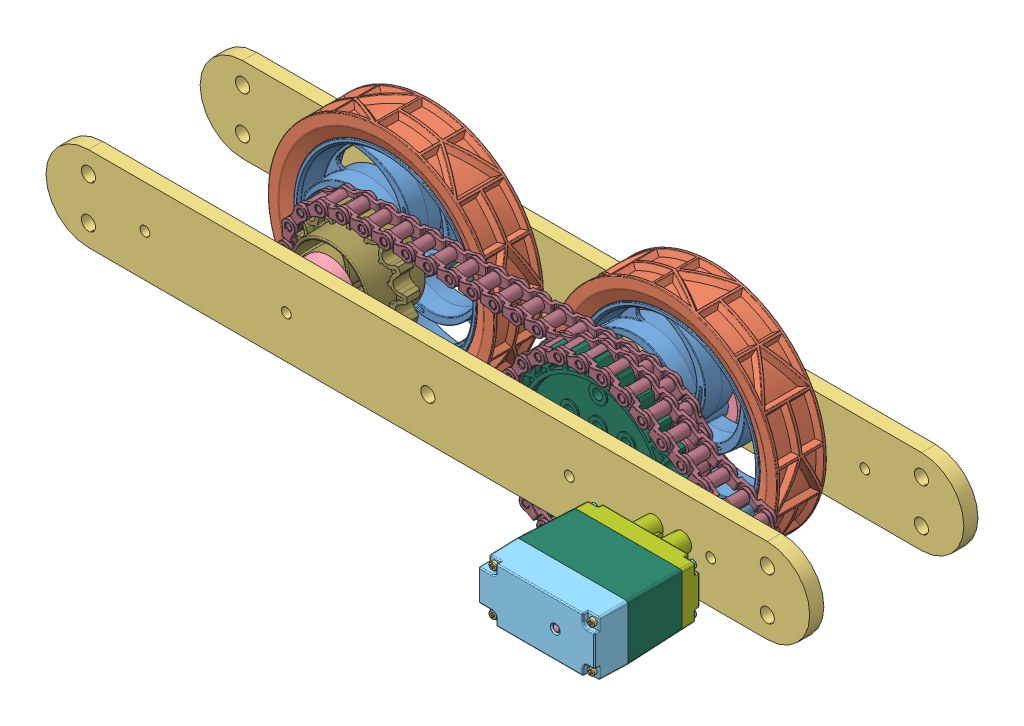
SolidWorks assembly WheelAssys, configuration Default. Lengths in mm.
Overall size (342.9 145.62 138.16).
125 component instances, 33 part files, 29 mates.
Components (placement in the parent):
- VEX-MEDIUM-WHEEL-3: VEX-MEDIUM-WHEEL [Default] at (104.6657 -17.1626 41.6298) x (-0.057006 -0.998374 0) z (0 0 1) size (152.02 138.56 24.07)
  - MEDIUM-WHEEL-HUB-1: MEDIUM-WHEEL-HUB [Default] at (-37.6569 24.2609 3.3885) size (92.9 92.77 19.05)
  - MEDIUM-WHEEL-TIRE-1: MEDIUM-WHEEL-TIRE [Default] at (-37.6569 24.2609 3.3885) x (-0.900891 -0.434045 0) z (-0.434045 0.900891 0) size (101.75 22.31 101.75)
- VEX-MEDIUM-WHEEL-4: VEX-MEDIUM-WHEEL [Default] at (294.9665 44.3997 41.6298) x (0.386599 0.922248 0) z (0 0 1) size (152.02 138.56 24.07)
  - MEDIUM-WHEEL-HUB-1: MEDIUM-WHEEL-HUB [Default] at (-37.6569 24.2609 3.3885) size (92.9 92.77 19.05)
  - MEDIUM-WHEEL-TIRE-1: MEDIUM-WHEEL-TIRE [Default] at (-37.6569 24.2609 3.3885) x (-0.900891 -0.434045 0) z (-0.434045 0.900891 0) size (101.75 22.31 101.75)
- sidebar-1: sidebar [Default] at (131.3771 19.05 23.1154) size (342.9 38.1 6.35)
- collar-2: collar [Default] at (131.0339 19.05 79.6212) x (0.952485 0.304585 0) z (0 0 1) size (25.4 25.4 6.35)
- DRIVE MOTOR-1: DRIVE MOTOR [Default] at (295.8339 19.05 146.6712) x (1 0 0) z (0 -1 0) size (56.4 63.4 25)
  - SPPM206-0150BO-1: SPPM206-0150BO [Default] at (-10.5 -23.5 -9.5) x (-1 0 0) z (0 0 1) size (3.3 16.36 3.3)
  - 276-2177-004 Rev1-1: 276-2177-004 Rev1 [Default] at (0 2.3 0) x (-0.521464 0 -0.853273) z (0 -1 0) size (5.83 5.83 4.5)
  - 276-2177-003 Rev1-1: 276-2177-003 Rev1 [Default] at (0 -25 0) size (48.69 26 23.69)
  - SPPM204-0050BO-1: SPPM204-0050BO [Default] at (0 -6.45 -6.2) size (3.3 6.41 3.3)
  - 276-2177-014 Rev1-1: 276-2177-014 Rev1 [Default] at (-11.6 -15 0) x (0 1 0) z (0 0 1) size (1 18.4 20.4)
  - 276-2177-005 Rev1-1: 276-2177-005 Rev1 [Default] at (12.1 2.15 0) x (-0.981818 0 0.189823) z (0 -1 0) size (19.95 19.95 7)
  - 276-2177-015 Rev2-1: 276-2177-015 Rev2 [Default] at (15.1 -10.55 0) x (-0.403604 0 0.914934) z (0 -1 0) size (14.01 14.03 13)
  - SPPM206-0150BO-2: SPPM206-0150BO [Default] at (33.5 -23.5 9.5) x (-1 0 0) z (0 0 1) size (3.3 16.36 3.3)
  - 276-2177-019 Rev1-1: 276-2177-019 Rev1 [Default] at (13 -33 0) x (0.158525 0 -0.987355) z (-0.987355 0 -0.158525) size (6.3 15.8 6.3)
  - 276-2177-016 Rev2-1: 276-2177-016 Rev2 [Default] at (25.7 -19.25 0) x (-0.479705 0 -0.87743) z (0 -1 0) size (15.08 15.08 17.5)
  - 276-2177-012 Rev1-1: 276-2177-012 Rev1 [Default] at (25.7 -19.1 0) x (-0.525336 0 0.850895) z (0 1 0) size (6 6 2.85)
  - 276-2177-002 Rev1-1: 276-2177-002 Rev1 [Default] at origin size (50 27.05 25)
  - LABLE_1-1: LABLE_1 [Default] at (27.1066 -2.1 2.9971) x (0.995174 0 0.098129) z (0 1 0) size (12 12 0.21)
  - 276-2177-011 Rev1-1: 276-2177-011 Rev1 [Default] at (12.1 -0.9 0) x (0 1 0) z (-0.101873 0 0.994797) size (14.8 2 2)
  - SPPM204-0050BO-2: SPPM204-0050BO [Default] at (0 -6.45 6.2) size (3.3 6.41 3.3)
  - FS130-FT-21100-1: FS130-FT-21100 [Default] at (0 -15 0) x (0 0 -1) z (0 1 0) size (20.4 15.4 34.7)
  - 276-2177-010 Rev1-1: 276-2177-010 Rev1 [Default] at (24.2 -4.9 0) x (0 1 0) z (0.653198 0 -0.757187) size (20.8 2 2)
  - 276-2177-006 Rev1-1: 276-2177-006 Rev1 [Default] at (24.2 -0.95 0) x (-0.999044 0 -0.043716) z (0 -1 0) size (20.25 20.26 13)
  - 276-1321-INST1-1: 276-1321-INST1 [Default] at origin size (52.31 18.11 25)
    - M2_1-1: M2_1 [Default] at (33.5 5 9.5) size (3.3 17.41 3.3)
    - LIGHT_1-1: LIGHT_1 [Default] at (-1.2 -1.6 0) x (-1 0 0) z (0 1 0) size (4.3 7.9 4.5)
    - M2_1-2: M2_1 [Default] at (-10.5 5 -9.5) size (3.3 17.41 3.3)
    - BOX-BOTTOM2_3-1: BOX-BOTTOM2_3 [Default] at origin size (52.31 14.6 25)
    - M2_1-3: M2_1 [Default] at (-10.5 5 9.5) size (3.3 17.41 3.3)
    - LABLE_1-1: LABLE_1 [Default] at (-3.1282 -2.1 -1.5101) x (-1 0 0) z (0 1 0) size (12 12 0.21)
    - M2_1-4: M2_1 [Default] at (33.5 5 -9.5) size (3.3 17.41 3.3)
    - PCB2_3-1: PCB2_3 [Default] at origin size (35.5 5.9 20)
    - PIN_ASM_1_ASM-1: PIN_ASM_1_ASM [Default] at (-2 9.01 -0.5) x (0 1 0) z (0 0 1) size (7.84 15.75 10.2)
      - PIN2_1-1: PIN2_1 [Default] at (2.62 -5.9 0) size (7.74 10.15 10.2)
      - PIN_1-1: PIN_1 [Default] at origin size (5.2 9.95 10.2)
  - 276-2177-019 Rev1-2: 276-2177-019 Rev1 [Default] at (0.3 -33 0) x (-0.999228 0 0.03928) z (0.03928 0 0.999228) size (6.3 15.8 6.3)
  - 276-2177-018 Rev1-1: 276-2177-018 Rev1 [Default] at (-12 2.1 0) x (0 0 -1) z (1 0 0) size (6.41 4.2 8.9)
  - SPPM206-0150BO-3: SPPM206-0150BO [Default] at (33.5 -23.5 -9.5) x (-1 0 0) z (0 0 1) size (3.3 16.36 3.3)
  - 276-2177-013 Rev1-1: 276-2177-013 Rev1 [Default] at (25.7 -31.5 0) x (-1 0 0) z (0 1 0) size (10 9.93 10.05)
  - SPPM206-0150BO-4: SPPM206-0150BO [Default] at (-10.5 -23.5 9.5) x (-1 0 0) z (0 0 1) size (3.3 16.36 3.3)
  - 276-2177-009 Rev1-1: 276-2177-009 Rev1 [Default] at (15.1 -17.75 0) x (1 0 0) z (0 -1 0) size (2 2 27.5)
- sprocket-1: sprocket [Default] at (258.0339 19.05 54.2212) x (0.004262 0.999991 0) z (0 0 1) size (50.77 50.68 25.4)
- sprocket-2: sprocket [Default] at (131.0339 19.05 54.2212) x (-0.057006 -0.998374 0) z (0 0 1) size (50.77 50.68 25.4)
- collar-5: collar [Default] at (131.0339 19.05 29.4654) x (0.952485 0.304585 0) z (0 0 1) size (25.4 25.4 6.35)
- collar-6: collar [Default] at (258.0339 19.05 29.4654) x (0.952485 0.304585 0) z (0 0 1) size (25.4 25.4 6.35)
- ChainLink-1: ChainLink [Default] at (267.9244 42.2656 63.5) x (0.826381 -0.563111 0) z (-0.563111 -0.826381 0) size (15.79 14.22 6)
- ChainLink-2: ChainLink [Default] at (258.3349 44.2828 63.5) x (0.978583 -0.205853 0) z (-0.205853 -0.978583 0) size (15.79 14.22 6)
- ChainLink-3: ChainLink [Default] at (248.5356 44.2846 63.5) x (1 -0.000183 0) z (-0.000183 -1 0) size (15.79 14.22 6)
- ChainLink-4: ChainLink [Default] at (238.7363 44.2846 63.5) x (1 0 0) z (0 -1 0) size (15.79 14.22 6)
- ChainLink-5: ChainLink [Default] at (228.9369 44.2846 63.5) x (1 0 0) z (0 -1 0) size (15.79 14.22 6)
- ChainLink-6: ChainLink [Default] at (219.1376 44.2846 63.5) x (1 0 0) z (0 -1 0) size (15.79 14.22 6)
- ChainLink-7: ChainLink [Default] at (209.3383 44.2846 63.5) x (1 0 0) z (0 -1 0) size (15.79 14.22 6)
- ChainLink-8: ChainLink [Default] at (199.539 44.2846 63.5) x (1 0 0) z (0 -1 0) size (15.79 14.22 6)
- ChainLink-9: ChainLink [Default] at (189.7397 44.2846 63.5) x (1 0 0) z (0 -1 0) size (15.79 14.22 6)
- ChainLink-10: ChainLink [Default] at (179.9403 44.2846 63.5) x (1 0 0) z (0 -1 0) size (15.79 14.22 6)
- ChainLink-11: ChainLink [Default] at (170.141 44.2846 63.5) x (1 0 0) z (0 -1 0) size (15.79 14.22 6)
- ChainLink-12: ChainLink [Default] at (160.3417 44.2846 63.5) x (1 0 0) z (0 -1 0) size (15.79 14.22 6)
- ChainLink-13: ChainLink [Default] at (150.5424 44.2846 63.5) x (1 0 0) z (0 -1 0) size (15.79 14.22 6)
- ChainLink-14: ChainLink [Default] at (140.7431 44.2846 63.5) x (1 0 0) z (0 -1 0) size (15.79 14.22 6)
- ChainLink-15: ChainLink [Default] at (130.9437 44.2845 63.5) x (1 0.000016 0) z (0.000016 -1 0) size (15.79 14.22 6)
- ChainLink-16: ChainLink [Default] at (121.3378 42.3475 63.5) x (0.980269 0.197666 0) z (0.197666 -0.980269 0) size (15.79 14.22 6)
- ChainLink-17: ChainLink [Default] at (113.194 36.8973 63.5) x (0.831059 0.556184 0) z (0.556184 -0.831059 0) size (15.79 14.22 6)
- ChainLink-18: ChainLink [Default] at (107.7404 28.7557 63.5) x (0.556526 0.83083 0) z (0.83083 -0.556526 0) size (15.79 14.22 6)
- ChainLink-19: ChainLink [Default] at (105.7994 19.1505 63.5) x (0.19807 0.980188 0) z (0.980188 -0.19807 0) size (15.79 14.22 6)
- ChainLink-20: ChainLink [Default] at (107.6638 9.5302 63.5) x (-0.190255 0.981735 0) z (0.981735 0.190255 0) size (15.79 14.22 6)
- ChainLink-21: ChainLink [Default] at (113.0524 1.3454 63.5) x (-0.54989 0.835237 0) z (0.835237 0.54989 0) size (15.79 14.22 6)
- ChainLink-22: ChainLink [Default] at (121.1525 -4.1695 63.5) x (-0.826602 0.562786 0) z (0.562786 0.826602 0) size (15.79 14.22 6)
- ChainLink-23: ChainLink [Default] at (130.7427 -6.183 63.5) x (-0.978664 0.205468 0) z (0.205468 0.978664 0) size (15.79 14.22 6)
- ChainLink-24: ChainLink [Default] at (140.5421 -6.1846 63.5) x (-1 0.000171 0) z (0.000171 1 0) size (15.79 14.22 6)
- ChainLink-25: ChainLink [Default] at (150.3414 -6.1846 63.5) x (-1 0 0) z (0 1 0) size (15.79 14.22 6)
- ChainLink-26: ChainLink [Default] at (160.1407 -6.1846 63.5) x (-1 0 0) z (0 1 0) size (15.79 14.22 6)
- ChainLink-27: ChainLink [Default] at (169.94 -6.1846 63.5) x (-1 0 0) z (0 1 0) size (15.79 14.22 6)
- ChainLink-28: ChainLink [Default] at (179.7393 -6.1846 63.5) x (-1 0 0) z (0 1 0) size (15.79 14.22 6)
- ChainLink-29: ChainLink [Default] at (189.5387 -6.1846 63.5) x (-1 0 0) z (0 1 0) size (15.79 14.22 6)
- ChainLink-30: ChainLink [Default] at (199.338 -6.1846 63.5) x (-1 0 0) z (0 1 0) size (15.79 14.22 6)
- ChainLink-31: ChainLink [Default] at (209.1373 -6.1846 63.5) x (-1 0 0) z (0 1 0) size (15.79 14.22 6)
- ChainLink-32: ChainLink [Default] at (218.9366 -6.1846 63.5) x (-1 0 0) z (0 1 0) size (15.79 14.22 6)
- ChainLink-33: ChainLink [Default] at (228.7359 -6.1846 63.5) x (-1 0 0) z (0 1 0) size (15.79 14.22 6)
- ChainLink-34: ChainLink [Default] at (238.5353 -6.1846 63.5) x (-1 0 0) z (0 1 0) size (15.79 14.22 6)
- ChainLink-35: ChainLink [Default] at (248.3346 -6.1846 63.5) x (-1 0 0) z (0 1 0) size (15.79 14.22 6)
- ChainLink-36: ChainLink [Default] at (258.1339 -6.1844 63.5) x (-1 -0.00002 0) z (-0.00002 1 0) size (15.79 14.22 6)
- ChainLink-37: ChainLink [Default] at (267.7391 -4.2437 63.5) x (-0.980192 -0.198051 0) z (-0.198051 0.980192 0) size (15.79 14.22 6)
- ChainLink-38: ChainLink [Default] at (275.8808 1.2098 63.5) x (-0.83084 -0.556511 0) z (-0.556511 0.83084 0) size (15.79 14.22 6)
- ChainLink-39: ChainLink [Default] at (281.3312 9.3535 63.5) x (-0.556199 -0.831049 0) z (-0.831049 0.556199 0) size (15.79 14.22 6)
- ChainLink-40: ChainLink [Default] at (283.2683 18.9594 63.5) x (-0.197684 -0.980266 0) z (-0.980266 0.197684 0) size (15.79 14.22 6)
- ChainLink-41: ChainLink [Default] at (281.4002 28.579 63.5) x (0.190641 -0.98166 0) z (-0.98166 -0.190641 0) size (15.79 14.22 6)
- ChainLink-44: ChainLink [Default] at (276.0084 36.7616 63.5) x (0.550219 -0.835021 0) z (-0.835021 -0.550219 0) size (15.79 14.22 6)
- 6-tooth-sprocket-1: 6-tooth-sprocket [Default] at (321.5339 19.05 84.3837) size (21.52 24.74 15.88)
- sidebar-5: sidebar [Default] at (131.3771 19.05 92.3212) size (342.9 38.1 6.35)
- collar-8: collar [Default] at (131.0339 19.05 85.9712) size (25.4 25.4 6.35)
- 24-tooth-sprocket-2: 24-tooth-sprocket [Default] at (258.0339 19.05 84.3837) size (80.15 80.15 15.88)
- ChainLink-45: ChainLink [Default] at (327.512 10.5358 88.5112) x (-0.891711 -0.452606 0) z (0.452606 -0.891711 0) size (15.79 14.22 6)
- ChainLink-46: ChainLink [Default] at (331.9347 19.2803 88.5112) x (-0.451325 -0.892359 0) z (0.892359 -0.451325 0) size (15.79 14.22 6)
- ChainLink-47: ChainLink [Default] at (327.1292 27.8205 88.5112) x (0.490382 -0.871507 0) z (0.871507 0.490382 0) size (15.79 14.22 6)
- ChainLink-48: ChainLink [Default] at (318.3636 32.2011 88.5112) x (0.894517 -0.447035 0) z (0.447035 0.894517 0) size (15.79 14.22 6)
- ChainLink-49: ChainLink [Default] at (309.5695 36.5244 88.5112) x (0.897416 -0.441185 0) z (0.441185 0.897416 0) size (15.79 14.22 6)
- ChainLink-50: ChainLink [Default] at (300.7755 40.8477 88.5112) x (0.897416 -0.441185 0) z (0.441185 0.897416 0) size (15.79 14.22 6)
- ChainLink-51: ChainLink [Default] at (291.9814 45.1711 88.5112) x (0.897416 -0.441185 0) z (0.441185 0.897416 0) size (15.79 14.22 6)
- ChainLink-52: ChainLink [Default] at (283.1873 49.4944 88.5112) x (0.897416 -0.441185 0) z (0.441185 0.897416 0) size (15.79 14.22 6)
- ChainLink-53: ChainLink [Default] at (274.3908 53.8126 88.5112) x (0.89767 -0.440669 0) z (0.440669 0.89767 0) size (15.79 14.22 6)
- ChainLink-54: ChainLink [Default] at (265.0643 56.8199 88.5112) x (0.951748 -0.306881 0) z (0.306881 0.951748 0) size (15.79 14.22 6)
- ChainLink-55: ChainLink [Default] at (255.2804 57.3698 88.5112) x (0.998424 -0.056121 0) z (0.056121 0.998424 0) size (15.79 14.22 6)
- ChainLink-56: ChainLink [Default] at (245.6757 55.4267 88.5112) x (0.980143 0.19829 0) z (-0.19829 0.980143 0) size (15.79 14.22 6)
- ChainLink-57: ChainLink [Default] at (236.875 51.117 88.5112) x (0.898096 0.4398 0) z (-0.4398 0.898096 0) size (15.79 14.22 6)
- ChainLink-58: ChainLink [Default] at (229.4508 44.721 88.5112) x (0.757618 0.652698 0) z (-0.652698 0.757618 0) size (15.79 14.22 6)
- ChainLink-59: ChainLink [Default] at (223.8863 36.6548 88.5112) x (0.567851 0.823131 0) z (-0.823131 0.567851 0) size (15.79 14.22 6)
- ChainLink-60: ChainLink [Default] at (220.5433 27.4434 88.5112) x (0.34114 0.940013 0) z (-0.940013 0.34114 0) size (15.79 14.22 6)
- ChainLink-61: ChainLink [Default] at (219.6395 17.6858 88.5112) x (0.092234 0.995737 0) z (-0.995737 0.092234 0) size (15.79 14.22 6)
- ChainLink-62: ChainLink [Default] at (221.2335 8.017 88.5112) x (-0.162672 0.98668 0) z (-0.98668 -0.162672 0) size (15.79 14.22 6)
- ChainLink-63: ChainLink [Default] at (225.2218 -0.934 88.5112) x (-0.406995 0.913431 0) z (-0.913431 -0.406995 0) size (15.79 14.22 6)
- ChainLink-64: ChainLink [Default] at (231.3448 -8.5848 88.5112) x (-0.624839 0.780754 0) z (-0.780754 -0.624839 0) size (15.79 14.22 6)
- ChainLink-65: ChainLink [Default] at (239.2042 -14.4378 88.5112) x (-0.802031 0.597282 0) z (-0.597282 -0.802031 0) size (15.79 14.22 6)
- ChainLink-66: ChainLink [Default] at (248.2886 -18.1121 88.5112) x (-0.927044 0.374951 0) z (-0.374951 -0.927044 0) size (15.79 14.22 6)
- ChainLink-67: ChainLink [Default] at (258.007 -19.3686 88.5112) x (-0.991745 0.128227 0) z (-0.128227 -0.991745 0) size (15.79 14.22 6)
- ChainLink-68: ChainLink [Default] at (267.7272 -18.1257 88.5112) x (-0.991923 -0.12684 0) z (0.12684 -0.991923 0) size (15.79 14.22 6)
- ChainLink-69: ChainLink [Default] at (276.8375 -14.5161 88.5112) x (-0.929687 -0.36835 0) z (0.36835 -0.929687 0) size (15.79 14.22 6)
- ChainLink-70: ChainLink [Default] at (285.6315 -10.1928 88.5112) x (-0.897416 -0.441185 0) z (0.441185 -0.897416 0) size (15.79 14.22 6)
- ChainLink-71: ChainLink [Default] at (294.4256 -5.8694 88.5112) x (-0.897416 -0.441185 0) z (0.441185 -0.897416 0) size (15.79 14.22 6)
- ChainLink-72: ChainLink [Default] at (303.2197 -1.5461 88.5112) x (-0.897416 -0.441185 0) z (0.441185 -0.897416 0) size (15.79 14.22 6)
- ChainLink-73: ChainLink [Default] at (312.0137 2.7772 88.5112) x (-0.897416 -0.441185 0) z (0.441185 -0.897416 0) size (15.79 14.22 6)
- ChainLink-74: ChainLink [Default] at (320.8078 7.1005 88.5112) x (-0.897416 -0.441185 0) z (0.441185 -0.897416 0) size (15.79 14.22 6)
Mates (geometry in assembly coordinates):
- Concentric13: concentric anti-aligned: circle of collar-2; circle of sprocket-2
- Coincident7: coincident anti-aligned: plane of collar-2 through (131.0339 19.05 79.6212) normal (0 0 -1); plane of sprocket-2 through (131.0339 19.05 79.6212) normal (0 0 1)
- Tangent9: tangent aligned: sphere of VEX-MEDIUM-WHEEL-3/MEDIUM-WHEEL-HUB-1; plane of sprocket-2 through (131.0339 19.05 54.2212) normal (0 0 -1)
- Concentric15: concentric anti-aligned: circle of VEX-MEDIUM-WHEEL-3/MEDIUM-WHEEL-HUB-1; circle of sprocket-2
- Tangent10: tangent aligned: sphere of VEX-MEDIUM-WHEEL-4/MEDIUM-WHEEL-HUB-1; plane of sprocket-1 through (258.0339 19.05 54.2212) normal (0 0 -1)
- Concentric16: concentric anti-aligned: circle of VEX-MEDIUM-WHEEL-4/MEDIUM-WHEEL-HUB-1; circle of sprocket-1
- Coincident8: coincident anti-aligned: plane of sidebar-1 through (42.1339 19.05 29.4654) normal (0 0 1); plane of collar-5 through (131.0339 19.05 29.4654) normal (0 0 -1)
- Concentric17: concentric aligned: cylinder of sidebar-1 through (131.0339 19.05 29.4654) axis (0 0 -1) radius 2.1828; cylinder of collar-5 through (131.0339 19.05 35.8154) axis (0 0 -1) radius 3.175
- Coincident9: coincident anti-aligned: plane of sidebar-1 through (42.1339 19.05 29.4654) normal (0 0 1); plane of collar-6 through (258.0339 19.05 29.4654) normal (0 0 -1)
- Concentric18: concentric aligned: cylinder of sidebar-1 through (258.0339 19.05 29.4654) axis (0 0 -1) radius 2.1828; cylinder of collar-6 through (258.0339 19.05 35.8154) axis (0 0 -1) radius 3.175
- Tangent11: tangent aligned: sphere of VEX-MEDIUM-WHEEL-3/MEDIUM-WHEEL-HUB-1; plane of collar-5 through (131.0339 19.05 35.8154) normal (0 0 1)
- Coincident15: coincident anti-aligned: plane of sidebar-1 through (42.1339 0 29.4654) normal (0 -1 0); plane of assembly through (0 0 0) normal (0 1 0)
- Lock5: lock: unknown of ?; unknown of sprocket-1
- Lock6: lock: unknown of ?; unknown of sprocket-2
- GearMate1: gear = 36.1991 : 36.1991 mm: circle of sprocket-1; circle of sprocket-2
- GearMate4: gear = 5.08 : 4.9987 mm: cylinder of ChainLink-14 through (140.7431 44.2846 71.5) axis (0 0 -1) radius 2.4994; cone of sprocket-2 through (131.0339 19.05 67.6712) axis (0 0 1)
- Coincident18: coincident aligned: circle of collar-2; circle of collar-8
- Coincident19: coincident anti-aligned: plane of sidebar-5 through (42.1339 19.05 92.3212) normal (0 0 -1); plane of collar-8 through (131.0339 19.05 92.3212) normal (0 0 1)
- Concentric20: concentric aligned: circle of sidebar-5; circle of collar-8
- Concentric22: concentric aligned: cylinder of sidebar-1 through (42.1339 28.575 29.4654) axis (0 0 -1) radius 3.175; cylinder of sidebar-5 through (42.1339 28.575 98.6712) axis (0 0 -1) radius 3.175
- Concentric23: concentric aligned: cylinder of sidebar-1 through (42.1339 9.525 29.4654) axis (0 0 -1) radius 3.175; cylinder of sidebar-5 through (42.1339 9.525 98.6712) axis (0 0 -1) radius 3.175
- Coincident21: coincident anti-aligned: plane of 6-tooth-sprocket-1 through (321.5339 19.05 92.3212) normal (0 0 1); plane of sidebar-5 through (42.1339 19.05 92.3212) normal (0 0 -1)
- Concentric24: concentric anti-aligned: circle of 6-tooth-sprocket-1; circle of sidebar-5
- Coincident22: coincident anti-aligned: plane of sidebar-5 through (42.1339 19.05 92.3212) normal (0 0 -1); plane of 24-tooth-sprocket-2 through (258.0339 19.05 92.3212) normal (0 0 1)
- Concentric25: concentric aligned: cylinder of sidebar-5 through (258.0339 19.05 98.6712) axis (0 0 -1) radius 2.1828; circle of 24-tooth-sprocket-2
- Lock7: lock: unknown of sidebar-1; unknown of sidebar-5
- Coincident24: coincident anti-aligned: plane of DRIVE MOTOR-1/276-2177-003 Rev1-1 through (295.8339 19.05 98.6712) normal (0 0 -1); plane of sidebar-5 through (42.1339 19.05 98.6712) normal (0 0 1)
- Parallel1: parallel anti-aligned: line of DRIVE MOTOR-1/276-2177-003 Rev1-1 through (283.9882 30.8954 121.6712) axis (1 0 0); line of sidebar-5 through (346.9339 38.1 98.6712) axis (-1 0 0)
- Concentric26: concentric aligned: circle of DRIVE MOTOR-1/276-2177-003 Rev1-1; circle of sidebar-5
